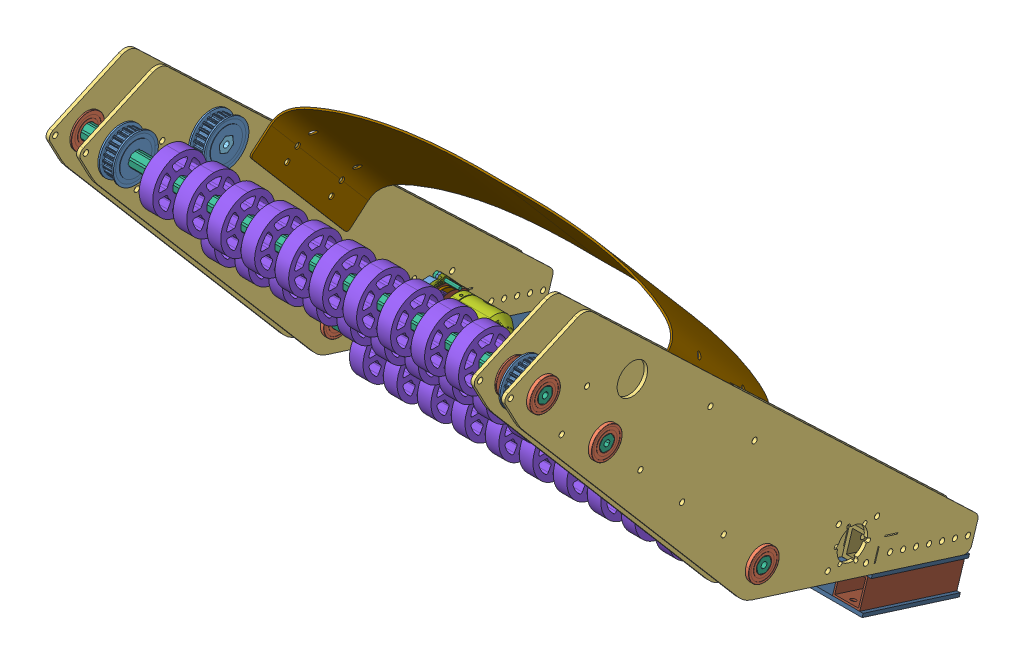
SolidWorks assembly 599-23-Prometheus-IntakeBackup-P-0000, configuration Default. Lengths in mm.
Overall size (438.38 502.65 458.04).
116 component instances, 30 part files, 15 mates.
Components (placement in the parent):
- EBUD-000_INTAKE_STEP_ASM^599-23-Prometheus-IntakeBackup-P-0000-1: EBUD-000_INTAKE_STEP_ASM^599-23-Prometheus-IntakeBackup-P-0000 [Default] at origin size (438.38 502.65 458.04) (virtual)
  - 24T_X_9MM_WIDE_DOUBLE_FLANGE_AL^EBUD-000_INTAKE_STEP_ASM_599-23-Prometheus-IntakeBackup-P-0000-1: 24T_X_9MM_WIDE_DOUBLE_FLANGE_AL^EBUD-000_INTAKE_STEP_ASM_599-23-Prometheus-IntakeBackup-P-0000 [Default] at (-209.55 741.6884 782.7658) x (0 0.711961 0.702219) z (1 0 0) size (42 42 14.5) (virtual)
  - 24T_X_9MM_WIDE_DOUBLE_FLANGE_AL^EBUD-000_INTAKE_STEP_ASM_599-23-Prometheus-IntakeBackup-P-0000-2: 24T_X_9MM_WIDE_DOUBLE_FLANGE_AL^EBUD-000_INTAKE_STEP_ASM_599-23-Prometheus-IntakeBackup-P-0000 [Default] at (-209.55 714.5782 696.9507) x (0 -0.172794 -0.984958) z (1 0 0) size (42 42 14.5) (virtual)
  - 13_75MM__1_2_THUNDERHEX_ID__X_1^EBUD-000_INTAKE_STEP_ASM_599-23-Prometheus-IntakeBackup-P-0000-1: 13_75MM__1_2_THUNDERHEX_ID__X_1^EBUD-000_INTAKE_STEP_ASM_599-23-Prometheus-IntakeBackup-P-0000 [Default] at (-224.6312 714.5782 696.9507) x (0 -0.939164 0.343468) z (1 0 0) size (31.12 31.12 7.94) (virtual)
  - 13_75MM__1_2_THUNDERHEX_ID__X_1^EBUD-000_INTAKE_STEP_ASM_599-23-Prometheus-IntakeBackup-P-0000-2: 13_75MM__1_2_THUNDERHEX_ID__X_1^EBUD-000_INTAKE_STEP_ASM_599-23-Prometheus-IntakeBackup-P-0000 [Default] at (-224.6312 741.6884 782.7658) x (0 -0.292473 -0.956274) z (1 0 0) size (31.12 31.12 7.94) (virtual)
  - 599-23-Prometheus-IntakeBackup-P-0004-1: 599-23-Prometheus-IntakeBackup-P-0004 [Default] at (-223.8375 981.3273 987.2051) x (1 0 0) z (0 -0.649023 0.760769) size (3.17 540.33 141.11)
  - 599-23-Prometheus-IntakeBackup-P-0004-2: 599-23-Prometheus-IntakeBackup-P-0004 [Default] at (-195.2625 981.3273 987.2051) x (1 0 0) z (0 -0.649023 0.760769) size (3.17 540.33 141.11)
  - 599-23-Prometheus-IntakeBackup-P-0004-3: 599-23-Prometheus-IntakeBackup-P-0004 [Default] at (173.1645 981.3273 987.2051) x (1 0 0) z (0 -0.649023 0.760769) size (3.17 540.33 141.11)
  - 599-23-Prometheus-IntakeBackup-P-0004-4: 599-23-Prometheus-IntakeBackup-P-0004 [Default] at (201.7395 981.3273 987.2051) x (1 0 0) z (0 -0.649023 0.760769) size (3.17 540.33 141.11)
  - 13_75MM__1_2_THUNDERHEX_ID__X_1^EBUD-000_INTAKE_STEP_ASM_599-23-Prometheus-IntakeBackup-P-0000-3: 13_75MM__1_2_THUNDERHEX_ID__X_1^EBUD-000_INTAKE_STEP_ASM_599-23-Prometheus-IntakeBackup-P-0000 [Default] at (-194.4688 981.3273 987.2051) x (0 0.254987 0.966944) z (-1 0 0) size (31.12 31.12 7.94) (virtual)
  - 13_75MM__1_2_THUNDERHEX_ID__X_1^EBUD-000_INTAKE_STEP_ASM_599-23-Prometheus-IntakeBackup-P-0000-4: 13_75MM__1_2_THUNDERHEX_ID__X_1^EBUD-000_INTAKE_STEP_ASM_599-23-Prometheus-IntakeBackup-P-0000 [Default] at (-224.6312 950.6568 902.5971) x (0 0.861369 0.50798) z (1 0 0) size (31.12 31.12 7.94) (virtual)
  - 13_75MM__1_2_THUNDERHEX_ID__X_1^EBUD-000_INTAKE_STEP_ASM_599-23-Prometheus-IntakeBackup-P-0000-5: 13_75MM__1_2_THUNDERHEX_ID__X_1^EBUD-000_INTAKE_STEP_ASM_599-23-Prometheus-IntakeBackup-P-0000 [Default] at (-224.6312 981.3273 987.2051) x (0 0.96991 0.243463) z (1 0 0) size (31.12 31.12 7.94) (virtual)
  - 24T_X_9MM_WIDE_DOUBLE_FLANGE_AL^EBUD-000_INTAKE_STEP_ASM_599-23-Prometheus-IntakeBackup-P-0000-3: 24T_X_9MM_WIDE_DOUBLE_FLANGE_AL^EBUD-000_INTAKE_STEP_ASM_599-23-Prometheus-IntakeBackup-P-0000 [Default] at (-183.25 981.3273 987.2051) x (0 -0.068988 0.997618) z (1 0 0) size (42 42 14.5) (virtual)
  - 13_75MM__1_2_THUNDERHEX_ID__X_1^EBUD-000_INTAKE_STEP_ASM_599-23-Prometheus-IntakeBackup-P-0000-6: 13_75MM__1_2_THUNDERHEX_ID__X_1^EBUD-000_INTAKE_STEP_ASM_599-23-Prometheus-IntakeBackup-P-0000 [Default] at (-194.4688 913.695 929.507) x (0 0.294166 0.955754) z (-1 0 0) size (31.12 31.12 7.94) (virtual)
  - 13_75MM__1_2_THUNDERHEX_ID__X_1^EBUD-000_INTAKE_STEP_ASM_599-23-Prometheus-IntakeBackup-P-0000-7: 13_75MM__1_2_THUNDERHEX_ID__X_1^EBUD-000_INTAKE_STEP_ASM_599-23-Prometheus-IntakeBackup-P-0000 [Default] at (-224.6312 913.695 929.507) x (0 0.91904 0.394165) z (1 0 0) size (31.12 31.12 7.94) (virtual)
  - REV-21-1929^EBUD-000_INTAKE_STEP_ASM_599-23-Prometheus-IntakeBackup-P-0000-1: REV-21-1929^EBUD-000_INTAKE_STEP_ASM_599-23-Prometheus-IntakeBackup-P-0000 [Default] at (-209.55 913.695 929.507) x (0 0 1) z (-1 0 0) size (48.2 48.2 12.7) (virtual)
  - 13_75MM__1_2_THUNDERHEX_ID__X_1^EBUD-000_INTAKE_STEP_ASM_599-23-Prometheus-IntakeBackup-P-0000-8: 13_75MM__1_2_THUNDERHEX_ID__X_1^EBUD-000_INTAKE_STEP_ASM_599-23-Prometheus-IntakeBackup-P-0000 [Default] at (-194.4688 741.6884 782.7658) x (0 -0.454664 -0.890663) z (-1 0 0) size (31.12 31.12 7.94) (virtual)
  - REV-21-1929^EBUD-000_INTAKE_STEP_ASM_599-23-Prometheus-IntakeBackup-P-0000-2: REV-21-1929^EBUD-000_INTAKE_STEP_ASM_599-23-Prometheus-IntakeBackup-P-0000 [Default] at (-209.55 950.6568 902.5971) x (0 0.397418 0.917638) z (-1 0 0) size (48.2 48.2 12.7) (virtual)
  - 13_75MM__1_2_THUNDERHEX_ID__X_1^EBUD-000_INTAKE_STEP_ASM_599-23-Prometheus-IntakeBackup-P-0000-9: 13_75MM__1_2_THUNDERHEX_ID__X_1^EBUD-000_INTAKE_STEP_ASM_599-23-Prometheus-IntakeBackup-P-0000 [Default] at (-194.4688 950.6568 902.5971) x (0 0.163432 0.986555) z (-1 0 0) size (31.12 31.12 7.94) (virtual)
  - 24T_X_9MM_WIDE_DOUBLE_FLANGE_AL^EBUD-000_INTAKE_STEP_ASM_599-23-Prometheus-IntakeBackup-P-0000-4: 24T_X_9MM_WIDE_DOUBLE_FLANGE_AL^EBUD-000_INTAKE_STEP_ASM_599-23-Prometheus-IntakeBackup-P-0000 [Default] at (-183.25 950.6568 902.5971) x (0 0.99517 0.098168) z (1 0 0) size (42 42 14.5) (virtual)
  - 13_75MM__1_2_THUNDERHEX_ID__X_1^EBUD-000_INTAKE_STEP_ASM_599-23-Prometheus-IntakeBackup-P-0000-10: 13_75MM__1_2_THUNDERHEX_ID__X_1^EBUD-000_INTAKE_STEP_ASM_599-23-Prometheus-IntakeBackup-P-0000 [Default] at (172.3707 913.695 929.507) x (0 -0.294166 -0.955754) z (1 0 0) size (31.12 31.12 7.94) (virtual)
  - 13_75MM__1_2_THUNDERHEX_ID__X_1^EBUD-000_INTAKE_STEP_ASM_599-23-Prometheus-IntakeBackup-P-0000-11: 13_75MM__1_2_THUNDERHEX_ID__X_1^EBUD-000_INTAKE_STEP_ASM_599-23-Prometheus-IntakeBackup-P-0000 [Default] at (172.3707 741.6884 782.7658) x (0 0.454664 0.890663) z (1 0 0) size (31.12 31.12 7.94) (virtual)
  - 13_75MM__1_2_THUNDERHEX_ID__X_1^EBUD-000_INTAKE_STEP_ASM_599-23-Prometheus-IntakeBackup-P-0000-12: 13_75MM__1_2_THUNDERHEX_ID__X_1^EBUD-000_INTAKE_STEP_ASM_599-23-Prometheus-IntakeBackup-P-0000 [Default] at (202.5333 981.3273 987.2051) x (0 -0.96991 -0.243463) z (-1 0 0) size (31.12 31.12 7.94) (virtual)
  - 13_75MM__1_2_THUNDERHEX_ID__X_1^EBUD-000_INTAKE_STEP_ASM_599-23-Prometheus-IntakeBackup-P-0000-13: 13_75MM__1_2_THUNDERHEX_ID__X_1^EBUD-000_INTAKE_STEP_ASM_599-23-Prometheus-IntakeBackup-P-0000 [Default] at (202.5333 913.695 929.507) x (0 -0.91904 -0.394165) z (-1 0 0) size (31.12 31.12 7.94) (virtual)
  - 13_75MM__1_2_THUNDERHEX_ID__X_1^EBUD-000_INTAKE_STEP_ASM_599-23-Prometheus-IntakeBackup-P-0000-14: 13_75MM__1_2_THUNDERHEX_ID__X_1^EBUD-000_INTAKE_STEP_ASM_599-23-Prometheus-IntakeBackup-P-0000 [Default] at (202.5333 741.6884 782.7658) x (0 0.292473 0.956274) z (-1 0 0) size (31.12 31.12 7.94) (virtual)
  - 13_75MM__1_2_THUNDERHEX_ID__X_1^EBUD-000_INTAKE_STEP_ASM_599-23-Prometheus-IntakeBackup-P-0000-15: 13_75MM__1_2_THUNDERHEX_ID__X_1^EBUD-000_INTAKE_STEP_ASM_599-23-Prometheus-IntakeBackup-P-0000 [Default] at (172.3707 981.3273 987.2051) x (0 -0.254987 -0.966944) z (1 0 0) size (31.12 31.12 7.94) (virtual)
  - 04_CLUSTER_SHAFT^EBUD-000_INTAKE_STEP_ASM_599-23-Prometheus-IntakeBackup-P-0000-1: 04_CLUSTER_SHAFT^EBUD-000_INTAKE_STEP_ASM_599-23-Prometheus-IntakeBackup-P-0000 [Default] at (-190.605 950.6568 902.5971) x (1 0 0) z (0 0.754856 0.65589) size (55.88 13.76 12.7) (virtual)
  - 24T_X_9MM_WIDE_DOUBLE_FLANGE_AL^EBUD-000_INTAKE_STEP_ASM_599-23-Prometheus-IntakeBackup-P-0000-5: 24T_X_9MM_WIDE_DOUBLE_FLANGE_AL^EBUD-000_INTAKE_STEP_ASM_599-23-Prometheus-IntakeBackup-P-0000 [Default] at (191.3145 741.6884 782.7658) x (0 -0.01901 0.999819) z (1 0 0) size (42 42 14.5) (virtual)
  - 24T_X_9MM_WIDE_DOUBLE_FLANGE_AL^EBUD-000_INTAKE_STEP_ASM_599-23-Prometheus-IntakeBackup-P-0000-6: 24T_X_9MM_WIDE_DOUBLE_FLANGE_AL^EBUD-000_INTAKE_STEP_ASM_599-23-Prometheus-IntakeBackup-P-0000 [Default] at (191.3145 981.3273 987.2051) x (0 -0.068988 0.997618) z (1 0 0) size (42 42 14.5) (virtual)
  - 04_INTAKE_ROLLER_SHAFT^EBUD-000_INTAKE_STEP_ASM_599-23-Prometheus-IntakeBackup-P-0000-1: 04_INTAKE_ROLLER_SHAFT^EBUD-000_INTAKE_STEP_ASM_599-23-Prometheus-IntakeBackup-P-0000 [Default] at (-37.973 741.6873 782.7662) x (1 0 0) z (0 -0.958269 0.285869) size (435.1 13.76 12.7) (virtual)
  - 04_INTAKE_ROLLER_SHAFT^EBUD-000_INTAKE_STEP_ASM_599-23-Prometheus-IntakeBackup-P-0000-2: 04_INTAKE_ROLLER_SHAFT^EBUD-000_INTAKE_STEP_ASM_599-23-Prometheus-IntakeBackup-P-0000 [Default] at (-37.973 913.695 929.507) x (1 0 0) z (0 -0.53426 -0.84532) size (435.1 13.76 12.7) (virtual)
  - 04_INTAKE_ROLLER_SHAFT^EBUD-000_INTAKE_STEP_ASM_599-23-Prometheus-IntakeBackup-P-0000-3: 04_INTAKE_ROLLER_SHAFT^EBUD-000_INTAKE_STEP_ASM_599-23-Prometheus-IntakeBackup-P-0000 [Default] at (-37.973 981.3273 987.2051) size (435.1 13.76 12.7) (virtual)
- REV_ULTRAPLANETARY_1-STAGE_ASM^599-23-Prometheus-IntakeBackup-P-0000-1: REV_ULTRAPLANETARY_1-STAGE_ASM^599-23-Prometheus-IntakeBackup-P-0000 [Default] at (-167.425 714.5782 696.9507) x (0 -0.976417 -0.215894) z (1 0 0) size (56.74 54.7 105.61) (virtual)
  - REV_ULTRAPLANETARY__CONFIGURABL_ASM^REV_ULTRAPLANETARY_1-STAGE_ASM_599-23-Prometheus-IntakeBackup-P-0000-1: REV_ULTRAPLANETARY__CONFIGURABL_ASM^REV_ULTRAPLANETARY_1-STAGE_ASM_599-23-Prometheus-IntakeBackup-P-0000 [Default] at origin size (56.74 54.7 105.61) (virtual)
    - REV_PLANETARY_STAGE__1__ASM^REV_ULTRAPLANETARY__CONFIGURABL_ASM_REV_ULTRAPLANETARY_1-STAGE_ASM_599-23-Prometheus-IntakeBackup-P-0000-1: REV_PLANETARY_STAGE__1__ASM^REV_ULTRAPLANETARY__CONFIGURABL_ASM_REV_ULTRAPLANETARY_1-STAGE_ASM_599-23-Prometheus-IntakeBackup-P-0000 [Default] at origin size (47.64 47.49 16.75) (virtual)
      - REV_ULTRAPLANETARY_3_1_CARTRIDG_ASM^REV_PLANETARY_STAGE__1__ASM_REV_ULTRAPLANETARY__CONFIGURABL_ASM_REV_ULTRAPLANETARY_1-STAGE_ASM_599-23-Prometheus-IntakeBackup-P-0000-1: REV_ULTRAPLANETARY_3_1_CARTRIDG_ASM^REV_PLANETARY_STAGE__1__ASM_REV_ULTRAPLANETARY__CONFIGURABL_ASM_REV_ULTRAPLANETARY_1-STAGE_ASM_599-23-Prometheus-IntakeBackup-P-0000 [Default] at origin size (47.64 47.49 16.75) (virtual)
        - REV-40-1613^REV_ULTRAPLANETARY_3_1_CARTRIDG_ASM_REV_PLANETARY_STAGE__1__ASM_REV_ULTRAPLANETARY__CONFIGURABL_ASM_REV_ULTRAPLANETARY_1-STAGE_ASM_599-23-Prometheus-IntakeBackup-P-0000-1: REV-40-1613^REV_ULTRAPLANETARY_3_1_CARTRIDG_ASM_REV_PLANETARY_STAGE__1__ASM_REV_ULTRAPLANETARY__CONFIGURABL_ASM_REV_ULTRAPLANETARY_1-STAGE_ASM_599-23-Prometheus-IntakeBackup-P-0000 [Default] at (-0.89 11.5157 -14.625) x (0 0 1) z (-0.923728 -0.383049 0) size (9 3 3) (virtual)
        - REV-41-1601-2^REV_ULTRAPLANETARY_3_1_CARTRIDG_ASM_REV_PLANETARY_STAGE__1__ASM_REV_ULTRAPLANETARY__CONFIGURABL_ASM_REV_ULTRAPLANETARY_1-STAGE_ASM_599-23-Prometheus-IntakeBackup-P-0000-1: REV-41-1601-2^REV_ULTRAPLANETARY_3_1_CARTRIDG_ASM_REV_PLANETARY_STAGE__1__ASM_REV_ULTRAPLANETARY__CONFIGURABL_ASM_REV_ULTRAPLANETARY_1-STAGE_ASM_599-23-Prometheus-IntakeBackup-P-0000 [Default] at (-0.89 11.5157 -8.625) x (0.281273 0.959628 0) z (0.959628 -0.281273 0) size (8.22 6.01 8.17) (virtual)
        - REV-41-1601-2^REV_ULTRAPLANETARY_3_1_CARTRIDG_ASM_REV_PLANETARY_STAGE__1__ASM_REV_ULTRAPLANETARY__CONFIGURABL_ASM_REV_ULTRAPLANETARY_1-STAGE_ASM_599-23-Prometheus-IntakeBackup-P-0000-2: REV-41-1601-2^REV_ULTRAPLANETARY_3_1_CARTRIDG_ASM_REV_PLANETARY_STAGE__1__ASM_REV_ULTRAPLANETARY__CONFIGURABL_ASM_REV_ULTRAPLANETARY_1-STAGE_ASM_599-23-Prometheus-IntakeBackup-P-0000 [Default] at (-11.5157 -0.89 -8.625) x (0.938661 0.34484 0) z (0.34484 -0.938661 0) size (8.22 6.01 8.17) (virtual)
        - REV-40-1613^REV_ULTRAPLANETARY_3_1_CARTRIDG_ASM_REV_PLANETARY_STAGE__1__ASM_REV_ULTRAPLANETARY__CONFIGURABL_ASM_REV_ULTRAPLANETARY_1-STAGE_ASM_599-23-Prometheus-IntakeBackup-P-0000-2: REV-40-1613^REV_ULTRAPLANETARY_3_1_CARTRIDG_ASM_REV_PLANETARY_STAGE__1__ASM_REV_ULTRAPLANETARY__CONFIGURABL_ASM_REV_ULTRAPLANETARY_1-STAGE_ASM_599-23-Prometheus-IntakeBackup-P-0000 [Default] at (0.89 -11.5157 -14.625) x (0 0 1) z (-0.923728 -0.383049 0) size (9 3 3) (virtual)
        - REV-40-1613^REV_ULTRAPLANETARY_3_1_CARTRIDG_ASM_REV_PLANETARY_STAGE__1__ASM_REV_ULTRAPLANETARY__CONFIGURABL_ASM_REV_ULTRAPLANETARY_1-STAGE_ASM_599-23-Prometheus-IntakeBackup-P-0000-3: REV-40-1613^REV_ULTRAPLANETARY_3_1_CARTRIDG_ASM_REV_PLANETARY_STAGE__1__ASM_REV_ULTRAPLANETARY__CONFIGURABL_ASM_REV_ULTRAPLANETARY_1-STAGE_ASM_599-23-Prometheus-IntakeBackup-P-0000 [Default] at (11.5157 0.89 -14.625) x (0 0 1) z (-0.923728 -0.383049 0) size (9 3 3) (virtual)
        - REV-41-1601-1^REV_ULTRAPLANETARY_3_1_CARTRIDG_ASM_REV_PLANETARY_STAGE__1__ASM_REV_ULTRAPLANETARY__CONFIGURABL_ASM_REV_ULTRAPLANETARY_1-STAGE_ASM_599-23-Prometheus-IntakeBackup-P-0000-1: REV-41-1601-1^REV_ULTRAPLANETARY_3_1_CARTRIDG_ASM_REV_PLANETARY_STAGE__1__ASM_REV_ULTRAPLANETARY__CONFIGURABL_ASM_REV_ULTRAPLANETARY_1-STAGE_ASM_599-23-Prometheus-IntakeBackup-P-0000 [Default] at (0 0 -11.875) x (0.997027 0.077058 0) z (0 0 -1) size (29.1 29.1 10.25) (virtual)
        - REV-41-1601-2^REV_ULTRAPLANETARY_3_1_CARTRIDG_ASM_REV_PLANETARY_STAGE__1__ASM_REV_ULTRAPLANETARY__CONFIGURABL_ASM_REV_ULTRAPLANETARY_1-STAGE_ASM_599-23-Prometheus-IntakeBackup-P-0000-3: REV-41-1601-2^REV_ULTRAPLANETARY_3_1_CARTRIDG_ASM_REV_PLANETARY_STAGE__1__ASM_REV_ULTRAPLANETARY__CONFIGURABL_ASM_REV_ULTRAPLANETARY_1-STAGE_ASM_599-23-Prometheus-IntakeBackup-P-0000 [Default] at (0.89 -11.5157 -8.625) x (0.79716 -0.603767 0) z (-0.603767 -0.79716 0) size (8.22 6.01 8.17) (virtual)
        - REV-41-1601-3^REV_ULTRAPLANETARY_3_1_CARTRIDG_ASM_REV_PLANETARY_STAGE__1__ASM_REV_ULTRAPLANETARY__CONFIGURABL_ASM_REV_ULTRAPLANETARY_1-STAGE_ASM_599-23-Prometheus-IntakeBackup-P-0000-1: REV-41-1601-3^REV_ULTRAPLANETARY_3_1_CARTRIDG_ASM_REV_PLANETARY_STAGE__1__ASM_REV_ULTRAPLANETARY__CONFIGURABL_ASM_REV_ULTRAPLANETARY_1-STAGE_ASM_599-23-Prometheus-IntakeBackup-P-0000 [Default] at (0 0 -8.75) x (-0.670912 -0.741537 0) z (-0.741537 0.670912 0) size (17.04 6.01 17.02) (virtual)
        - REV-40-1619^REV_ULTRAPLANETARY_3_1_CARTRIDG_ASM_REV_PLANETARY_STAGE__1__ASM_REV_ULTRAPLANETARY__CONFIGURABL_ASM_REV_ULTRAPLANETARY_1-STAGE_ASM_599-23-Prometheus-IntakeBackup-P-0000-1: REV-40-1619^REV_ULTRAPLANETARY_3_1_CARTRIDG_ASM_REV_PLANETARY_STAGE__1__ASM_REV_ULTRAPLANETARY__CONFIGURABL_ASM_REV_ULTRAPLANETARY_1-STAGE_ASM_599-23-Prometheus-IntakeBackup-P-0000 [Default] at (0 0 -14.875) x (-0.866025 -0.5 0) z (0 0 -1) size (35.02 34.62 3.62) (virtual)
        - REV-40-1619^REV_ULTRAPLANETARY_3_1_CARTRIDG_ASM_REV_PLANETARY_STAGE__1__ASM_REV_ULTRAPLANETARY__CONFIGURABL_ASM_REV_ULTRAPLANETARY_1-STAGE_ASM_599-23-Prometheus-IntakeBackup-P-0000-2: REV-40-1619^REV_ULTRAPLANETARY_3_1_CARTRIDG_ASM_REV_PLANETARY_STAGE__1__ASM_REV_ULTRAPLANETARY__CONFIGURABL_ASM_REV_ULTRAPLANETARY_1-STAGE_ASM_599-23-Prometheus-IntakeBackup-P-0000 [Default] at (0 0 -5.125) x (0 -1 0) z (0 0 1) size (35.02 34.62 3.62) (virtual)
        - REV-40-1613^REV_ULTRAPLANETARY_3_1_CARTRIDG_ASM_REV_PLANETARY_STAGE__1__ASM_REV_ULTRAPLANETARY__CONFIGURABL_ASM_REV_ULTRAPLANETARY_1-STAGE_ASM_599-23-Prometheus-IntakeBackup-P-0000-4: REV-40-1613^REV_ULTRAPLANETARY_3_1_CARTRIDG_ASM_REV_PLANETARY_STAGE__1__ASM_REV_ULTRAPLANETARY__CONFIGURABL_ASM_REV_ULTRAPLANETARY_1-STAGE_ASM_599-23-Prometheus-IntakeBackup-P-0000 [Default] at (-11.5157 -0.89 -14.625) x (0 0 1) z (-0.923728 -0.383049 0) size (9 3 3) (virtual)
        - REV-41-1601-2^REV_ULTRAPLANETARY_3_1_CARTRIDG_ASM_REV_PLANETARY_STAGE__1__ASM_REV_ULTRAPLANETARY__CONFIGURABL_ASM_REV_ULTRAPLANETARY_1-STAGE_ASM_599-23-Prometheus-IntakeBackup-P-0000-4: REV-41-1601-2^REV_ULTRAPLANETARY_3_1_CARTRIDG_ASM_REV_PLANETARY_STAGE__1__ASM_REV_ULTRAPLANETARY__CONFIGURABL_ASM_REV_ULTRAPLANETARY_1-STAGE_ASM_599-23-Prometheus-IntakeBackup-P-0000 [Default] at (11.5157 0.89 -8.625) x (0.79726 -0.603636 0) z (-0.603636 -0.79726 0) size (8.22 6.01 8.17) (virtual)
    - REV_ULTRAPLANETARY_OUTPUT_STAGE_ASM^REV_ULTRAPLANETARY__CONFIGURABL_ASM_REV_ULTRAPLANETARY_1-STAGE_ASM_599-23-Prometheus-IntakeBackup-P-0000-1: REV_ULTRAPLANETARY_OUTPUT_STAGE_ASM^REV_ULTRAPLANETARY__CONFIGURABL_ASM_REV_ULTRAPLANETARY_1-STAGE_ASM_599-23-Prometheus-IntakeBackup-P-0000 [Default] at origin size (56.74 54.7 18.3) (virtual)
      - REV-41-1604-5^REV_ULTRAPLANETARY_OUTPUT_STAGE_ASM_REV_ULTRAPLANETARY__CONFIGURABL_ASM_REV_ULTRAPLANETARY_1-STAGE_ASM_599-23-Prometheus-IntakeBackup-P-0000-1: REV-41-1604-5^REV_ULTRAPLANETARY_OUTPUT_STAGE_ASM_REV_ULTRAPLANETARY__CONFIGURABL_ASM_REV_ULTRAPLANETARY_1-STAGE_ASM_599-23-Prometheus-IntakeBackup-P-0000 [Default] at (0 0 -21.25) x (0.103978 -0.99458 0) z (0.99458 0.103978 0) size (23.5 0.75 23.5) (virtual)
      - SOCKET_HEAD_CAP_SCREW_AM_B18_3_^REV_ULTRAPLANETARY_OUTPUT_STAGE_ASM_REV_ULTRAPLANETARY__CONFIGURABL_ASM_REV_ULTRAPLANETARY_1-STAGE_ASM_599-23-Prometheus-IntakeBackup-P-0000-1: SOCKET_HEAD_CAP_SCREW_AM_B18_3_^REV_ULTRAPLANETARY_OUTPUT_STAGE_ASM_REV_ULTRAPLANETARY__CONFIGURABL_ASM_REV_ULTRAPLANETARY_1-STAGE_ASM_599-23-Prometheus-IntakeBackup-P-0000 [Default] at (15.6357 3.3948 -15.05) x (0 0 -1) z (-0.934724 -0.355374 0) size (6 3.8 3.8) (virtual)
      - MCMASTER-CARR_91292A004_91292A0^REV_ULTRAPLANETARY_OUTPUT_STAGE_ASM_REV_ULTRAPLANETARY__CONFIGURABL_ASM_REV_ULTRAPLANETARY_1-STAGE_ASM_599-23-Prometheus-IntakeBackup-P-0000-1: MCMASTER-CARR_91292A004_91292A0^REV_ULTRAPLANETARY_OUTPUT_STAGE_ASM_REV_ULTRAPLANETARY__CONFIGURABL_ASM_REV_ULTRAPLANETARY_1-STAGE_ASM_599-23-Prometheus-IntakeBackup-P-0000 [Default] at (-3.715 6.4346 -21.5) x (-0.608447 -0.793594 0) z (-0.793594 0.608447 0) size (3.8 6 3.8) (virtual)
      - 6704ZZ^REV_ULTRAPLANETARY_OUTPUT_STAGE_ASM_REV_ULTRAPLANETARY__CONFIGURABL_ASM_REV_ULTRAPLANETARY_1-STAGE_ASM_599-23-Prometheus-IntakeBackup-P-0000-1: 6704ZZ^REV_ULTRAPLANETARY_OUTPUT_STAGE_ASM_REV_ULTRAPLANETARY__CONFIGURABL_ASM_REV_ULTRAPLANETARY_1-STAGE_ASM_599-23-Prometheus-IntakeBackup-P-0000 [Default] at (0 0 -23.25) x (0.117109 -0.993119 0) z (0.993119 0.117109 0) size (27 4 27) (virtual)
      - 6704ZZ^REV_ULTRAPLANETARY_OUTPUT_STAGE_ASM_REV_ULTRAPLANETARY__CONFIGURABL_ASM_REV_ULTRAPLANETARY_1-STAGE_ASM_599-23-Prometheus-IntakeBackup-P-0000-2: 6704ZZ^REV_ULTRAPLANETARY_OUTPUT_STAGE_ASM_REV_ULTRAPLANETARY__CONFIGURABL_ASM_REV_ULTRAPLANETARY_1-STAGE_ASM_599-23-Prometheus-IntakeBackup-P-0000 [Default] at (0 0 -18.5) x (-0.099871 -0.995 0) z (0.995 -0.099871 0) size (27 4 27) (virtual)
      - MCMASTER-CARR_91292A004_91292A0^REV_ULTRAPLANETARY_OUTPUT_STAGE_ASM_REV_ULTRAPLANETARY__CONFIGURABL_ASM_REV_ULTRAPLANETARY_1-STAGE_ASM_599-23-Prometheus-IntakeBackup-P-0000-2: MCMASTER-CARR_91292A004_91292A0^REV_ULTRAPLANETARY_OUTPUT_STAGE_ASM_REV_ULTRAPLANETARY__CONFIGURABL_ASM_REV_ULTRAPLANETARY_1-STAGE_ASM_599-23-Prometheus-IntakeBackup-P-0000 [Default] at (-3.715 -6.4346 -21.5) x (0.991496 -0.130134 0) z (-0.130134 -0.991496 0) size (3.8 6 3.8) (virtual)
      - MCMASTER-CARR_91292A004_91292A0^REV_ULTRAPLANETARY_OUTPUT_STAGE_ASM_REV_ULTRAPLANETARY__CONFIGURABL_ASM_REV_ULTRAPLANETARY_1-STAGE_ASM_599-23-Prometheus-IntakeBackup-P-0000-3: MCMASTER-CARR_91292A004_91292A0^REV_ULTRAPLANETARY_OUTPUT_STAGE_ASM_REV_ULTRAPLANETARY__CONFIGURABL_ASM_REV_ULTRAPLANETARY_1-STAGE_ASM_599-23-Prometheus-IntakeBackup-P-0000 [Default] at (7.43 0 -21.5) x (-0.383049 0.923728 0) z (0.923728 0.383049 0) size (3.8 6 3.8) (virtual)
      - SOCKET_HEAD_CAP_SCREW_AM_B18_3_^REV_ULTRAPLANETARY_OUTPUT_STAGE_ASM_REV_ULTRAPLANETARY__CONFIGURABL_ASM_REV_ULTRAPLANETARY_1-STAGE_ASM_599-23-Prometheus-IntakeBackup-P-0000-2: SOCKET_HEAD_CAP_SCREW_AM_B18_3_^REV_ULTRAPLANETARY_OUTPUT_STAGE_ASM_REV_ULTRAPLANETARY__CONFIGURABL_ASM_REV_ULTRAPLANETARY_1-STAGE_ASM_599-23-Prometheus-IntakeBackup-P-0000 [Default] at (-10.7579 11.8435 -15.05) x (0 0 -1) z (-0.492915 -0.870077 0) size (6 3.8 3.8) (virtual)
      - REV-41-1604-2^REV_ULTRAPLANETARY_OUTPUT_STAGE_ASM_REV_ULTRAPLANETARY__CONFIGURABL_ASM_REV_ULTRAPLANETARY_1-STAGE_ASM_599-23-Prometheus-IntakeBackup-P-0000-1: REV-41-1604-2^REV_ULTRAPLANETARY_OUTPUT_STAGE_ASM_REV_ULTRAPLANETARY__CONFIGURABL_ASM_REV_ULTRAPLANETARY_1-STAGE_ASM_599-23-Prometheus-IntakeBackup-P-0000 [Default] at (0 0 -26.25) x (0 -1 0) z (1 0 0) size (43.57 6.3 38.01) (virtual)
      - REV-41-1611_THROUGH_HOLE^REV_ULTRAPLANETARY_OUTPUT_STAGE_ASM_REV_ULTRAPLANETARY__CONFIGURABL_ASM_REV_ULTRAPLANETARY_1-STAGE_ASM_599-23-Prometheus-IntakeBackup-P-0000-1: REV-41-1611_THROUGH_HOLE^REV_ULTRAPLANETARY_OUTPUT_STAGE_ASM_REV_ULTRAPLANETARY__CONFIGURABL_ASM_REV_ULTRAPLANETARY_1-STAGE_ASM_599-23-Prometheus-IntakeBackup-P-0000 [Default] at (0 0 -15.25) x (0 1 0) z (1 0 0) size (22 6.76 22) (virtual)
      - REV-41-1612^REV_ULTRAPLANETARY_OUTPUT_STAGE_ASM_REV_ULTRAPLANETARY__CONFIGURABL_ASM_REV_ULTRAPLANETARY_1-STAGE_ASM_599-23-Prometheus-IntakeBackup-P-0000-1: REV-41-1612^REV_ULTRAPLANETARY_OUTPUT_STAGE_ASM_REV_ULTRAPLANETARY__CONFIGURABL_ASM_REV_ULTRAPLANETARY_1-STAGE_ASM_599-23-Prometheus-IntakeBackup-P-0000 [Default] at (0 0 -19) x (-0.5 -0.866025 0) z (0 0 -1) size (22 21.65 13.25) (virtual)
      - REV-41-1604-1^REV_ULTRAPLANETARY_OUTPUT_STAGE_ASM_REV_ULTRAPLANETARY__CONFIGURABL_ASM_REV_ULTRAPLANETARY_1-STAGE_ASM_599-23-Prometheus-IntakeBackup-P-0000-1: REV-41-1604-1^REV_ULTRAPLANETARY_OUTPUT_STAGE_ASM_REV_ULTRAPLANETARY__CONFIGURABL_ASM_REV_ULTRAPLANETARY_1-STAGE_ASM_599-23-Prometheus-IntakeBackup-P-0000 [Default] at (0 0 -19.25) x (0.866025 -0.5 0) z (-0.5 -0.866025 0) size (43.57 7.04 38.01) (virtual)
      - SOCKET_HEAD_CAP_SCREW_AM_B18_3_^REV_ULTRAPLANETARY_OUTPUT_STAGE_ASM_REV_ULTRAPLANETARY__CONFIGURABL_ASM_REV_ULTRAPLANETARY_1-STAGE_ASM_599-23-Prometheus-IntakeBackup-P-0000-3: SOCKET_HEAD_CAP_SCREW_AM_B18_3_^REV_ULTRAPLANETARY_OUTPUT_STAGE_ASM_REV_ULTRAPLANETARY__CONFIGURABL_ASM_REV_ULTRAPLANETARY_1-STAGE_ASM_599-23-Prometheus-IntakeBackup-P-0000 [Default] at (-4.8778 -15.2383 -15.05) x (0 0 -1) z (0.970727 -0.240185 0) size (6 3.8 3.8) (virtual)
    - REV_ULTRAPLANETARY_550_MOTOR_PL_ASM^REV_ULTRAPLANETARY__CONFIGURABL_ASM_REV_ULTRAPLANETARY_1-STAGE_ASM_599-23-Prometheus-IntakeBackup-P-0000-1: REV_ULTRAPLANETARY_550_MOTOR_PL_ASM^REV_ULTRAPLANETARY__CONFIGURABL_ASM_REV_ULTRAPLANETARY_1-STAGE_ASM_599-23-Prometheus-IntakeBackup-P-0000 [Default] at origin size (9.12 31.6 16.65) (virtual)
      - REV-41-1608^REV_ULTRAPLANETARY_550_MOTOR_PL_ASM_REV_ULTRAPLANETARY__CONFIGURABL_ASM_REV_ULTRAPLANETARY_1-STAGE_ASM_599-23-Prometheus-IntakeBackup-P-0000-1: REV-41-1608^REV_ULTRAPLANETARY_550_MOTOR_PL_ASM_REV_ULTRAPLANETARY__CONFIGURABL_ASM_REV_ULTRAPLANETARY_1-STAGE_ASM_599-23-Prometheus-IntakeBackup-P-0000 [Default] at (0 0 -8) x (-0.123066 0.992399 0) z (0.992399 0.123066 0) size (8.22 7 8.17) (virtual)
      - M3X8_BUTTON_HEAD_91239A113^REV_ULTRAPLANETARY_550_MOTOR_PL_ASM_REV_ULTRAPLANETARY__CONFIGURABL_ASM_REV_ULTRAPLANETARY_1-STAGE_ASM_599-23-Prometheus-IntakeBackup-P-0000-1: M3X8_BUTTON_HEAD_91239A113^REV_ULTRAPLANETARY_550_MOTOR_PL_ASM_REV_ULTRAPLANETARY__CONFIGURABL_ASM_REV_ULTRAPLANETARY_1-STAGE_ASM_599-23-Prometheus-IntakeBackup-P-0000 [Default] at (0.5 -12.49 -4.5) x (-0.04 0.9992 0) z (0.9992 0.04 0) size (5.7 9.66 5.7) (virtual)
      - M3X8_BUTTON_HEAD_91239A113^REV_ULTRAPLANETARY_550_MOTOR_PL_ASM_REV_ULTRAPLANETARY__CONFIGURABL_ASM_REV_ULTRAPLANETARY_1-STAGE_ASM_599-23-Prometheus-IntakeBackup-P-0000-2: M3X8_BUTTON_HEAD_91239A113^REV_ULTRAPLANETARY_550_MOTOR_PL_ASM_REV_ULTRAPLANETARY__CONFIGURABL_ASM_REV_ULTRAPLANETARY_1-STAGE_ASM_599-23-Prometheus-IntakeBackup-P-0000 [Default] at (-0.5 12.49 -4.5) x (-0.938759 0.344575 0) z (0.344575 0.938759 0) size (5.7 9.66 5.7) (virtual)
    - HEX_SOCKET_HEAD_CAP_SCREW_M3X0_^REV_ULTRAPLANETARY__CONFIGURABL_ASM_REV_ULTRAPLANETARY_1-STAGE_ASM_599-23-Prometheus-IntakeBackup-P-0000-1: HEX_SOCKET_HEAD_CAP_SCREW_M3X0_^REV_ULTRAPLANETARY__CONFIGURABL_ASM_REV_ULTRAPLANETARY_1-STAGE_ASM_599-23-Prometheus-IntakeBackup-P-0000 [Default] at (6.9282 4 -38.25) x (-0.866025 0.5 0) z (0 0 -1) size (5.5 5.5 11) (virtual)
    - HEX_SOCKET_HEAD_CAP_SCREW_M3X0_^REV_ULTRAPLANETARY__CONFIGURABL_ASM_REV_ULTRAPLANETARY_1-STAGE_ASM_599-23-Prometheus-IntakeBackup-P-0000-2: HEX_SOCKET_HEAD_CAP_SCREW_M3X0_^REV_ULTRAPLANETARY__CONFIGURABL_ASM_REV_ULTRAPLANETARY_1-STAGE_ASM_599-23-Prometheus-IntakeBackup-P-0000 [Default] at (0 8 -38.25) x (-0.866025 -0.5 0) z (0 0 -1) size (5.5 5.5 11) (virtual)
    - UP_1_2__HEX_ADAPTER__REV-41-162^REV_ULTRAPLANETARY__CONFIGURABL_ASM_REV_ULTRAPLANETARY_1-STAGE_ASM_599-23-Prometheus-IntakeBackup-P-0000-1: UP_1_2__HEX_ADAPTER__REV-41-162^REV_ULTRAPLANETARY__CONFIGURABL_ASM_REV_ULTRAPLANETARY_1-STAGE_ASM_599-23-Prometheus-IntakeBackup-P-0000 [Default] at (0 0 -32.25) x (-0.5 -0.866025 0) z (0 0 1) size (22 22 30.59) (virtual)
    - HEX_SOCKET_HEAD_CAP_SCREW_M3X0_^REV_ULTRAPLANETARY__CONFIGURABL_ASM_REV_ULTRAPLANETARY_1-STAGE_ASM_599-23-Prometheus-IntakeBackup-P-0000-3: HEX_SOCKET_HEAD_CAP_SCREW_M3X0_^REV_ULTRAPLANETARY__CONFIGURABL_ASM_REV_ULTRAPLANETARY_1-STAGE_ASM_599-23-Prometheus-IntakeBackup-P-0000 [Default] at (0 -8 -38.25) x (0.866025 0.5 0) z (0 0 -1) size (5.5 5.5 11) (virtual)
    - HEX_SOCKET_HEAD_CAP_SCREW_M3X0_^REV_ULTRAPLANETARY__CONFIGURABL_ASM_REV_ULTRAPLANETARY_1-STAGE_ASM_599-23-Prometheus-IntakeBackup-P-0000-4: HEX_SOCKET_HEAD_CAP_SCREW_M3X0_^REV_ULTRAPLANETARY__CONFIGURABL_ASM_REV_ULTRAPLANETARY_1-STAGE_ASM_599-23-Prometheus-IntakeBackup-P-0000 [Default] at (-6.9282 -4 -38.25) x (0.866025 -0.5 0) z (0 0 -1) size (5.5 5.5 11) (virtual)
    - M3X40_91290A136^REV_ULTRAPLANETARY__CONFIGURABL_ASM_REV_ULTRAPLANETARY_1-STAGE_ASM_599-23-Prometheus-IntakeBackup-P-0000-1: M3X40_91290A136^REV_ULTRAPLANETARY__CONFIGURABL_ASM_REV_ULTRAPLANETARY_1-STAGE_ASM_599-23-Prometheus-IntakeBackup-P-0000 [Default] at (0 18.4752 18.75) x (-0.866025 0.5 0) z (-0.5 -0.866025 0) size (5.5 23.01 5.5) (virtual)
    - M3X40_91290A136^REV_ULTRAPLANETARY__CONFIGURABL_ASM_REV_ULTRAPLANETARY_1-STAGE_ASM_599-23-Prometheus-IntakeBackup-P-0000-2: M3X40_91290A136^REV_ULTRAPLANETARY__CONFIGURABL_ASM_REV_ULTRAPLANETARY_1-STAGE_ASM_599-23-Prometheus-IntakeBackup-P-0000 [Default] at (-16 9.2376 18.75) x (-0.866025 -0.5 0) z (0.5 -0.866025 0) size (5.5 23.01 5.5) (virtual)
    - M3X40_91290A136^REV_ULTRAPLANETARY__CONFIGURABL_ASM_REV_ULTRAPLANETARY_1-STAGE_ASM_599-23-Prometheus-IntakeBackup-P-0000-3: M3X40_91290A136^REV_ULTRAPLANETARY__CONFIGURABL_ASM_REV_ULTRAPLANETARY_1-STAGE_ASM_599-23-Prometheus-IntakeBackup-P-0000 [Default] at (16 -9.2376 18.75) x (0.866025 0.5 0) z (-0.5 0.866025 0) size (5.5 23.01 5.5) (virtual)
    - HEX_SOCKET_HEAD_CAP_SCREW_M3X0_^REV_ULTRAPLANETARY__CONFIGURABL_ASM_REV_ULTRAPLANETARY_1-STAGE_ASM_599-23-Prometheus-IntakeBackup-P-0000-5: HEX_SOCKET_HEAD_CAP_SCREW_M3X0_^REV_ULTRAPLANETARY__CONFIGURABL_ASM_REV_ULTRAPLANETARY_1-STAGE_ASM_599-23-Prometheus-IntakeBackup-P-0000 [Default] at (6.9282 -4 -38.25) x (0 1 0) z (0 0 -1) size (5.5 5.5 11) (virtual)
    - M3X40_91290A136^REV_ULTRAPLANETARY__CONFIGURABL_ASM_REV_ULTRAPLANETARY_1-STAGE_ASM_599-23-Prometheus-IntakeBackup-P-0000-4: M3X40_91290A136^REV_ULTRAPLANETARY__CONFIGURABL_ASM_REV_ULTRAPLANETARY_1-STAGE_ASM_599-23-Prometheus-IntakeBackup-P-0000 [Default] at (-16 -9.2376 18.75) x (0 -1 0) z (1 0 0) size (5.5 23.01 5.5) (virtual)
    - M3X40_91290A136^REV_ULTRAPLANETARY__CONFIGURABL_ASM_REV_ULTRAPLANETARY_1-STAGE_ASM_599-23-Prometheus-IntakeBackup-P-0000-5: M3X40_91290A136^REV_ULTRAPLANETARY__CONFIGURABL_ASM_REV_ULTRAPLANETARY_1-STAGE_ASM_599-23-Prometheus-IntakeBackup-P-0000 [Default] at (0 -18.4752 18.75) x (0.866025 -0.5 0) z (0.5 0.866025 0) size (5.5 23.01 5.5) (virtual)
    - M3X40_91290A136^REV_ULTRAPLANETARY__CONFIGURABL_ASM_REV_ULTRAPLANETARY_1-STAGE_ASM_599-23-Prometheus-IntakeBackup-P-0000-6: M3X40_91290A136^REV_ULTRAPLANETARY__CONFIGURABL_ASM_REV_ULTRAPLANETARY_1-STAGE_ASM_599-23-Prometheus-IntakeBackup-P-0000 [Default] at (16 9.2376 18.75) x (0 1 0) z (-1 0 0) size (5.5 23.01 5.5) (virtual)
    - NEO_550_MOTOR__REV-21-1651_^REV_ULTRAPLANETARY__CONFIGURABL_ASM_REV_ULTRAPLANETARY_1-STAGE_ASM_599-23-Prometheus-IntakeBackup-P-0000-1: NEO_550_MOTOR__REV-21-1651_^REV_ULTRAPLANETARY__CONFIGURABL_ASM_REV_ULTRAPLANETARY_1-STAGE_ASM_599-23-Prometheus-IntakeBackup-P-0000 [Default] at (0 0 -11.5) x (0 0 1) z (-1 0 0) size (56.02 43 42.91) (virtual)
- TTB-0032_2INCH_SQUISH_WHEEL^599-23-Prometheus-IntakeBackup-P-0000-1: TTB-0032_2INCH_SQUISH_WHEEL^599-23-Prometheus-IntakeBackup-P-0000 [Default] at (143.002 741.6873 782.7662) x (0 0.999841 0.017831) z (0 -0.017831 0.999841) size (50.8 12.7 50.8) (virtual)
- TTB-0032_2INCH_SQUISH_WHEEL^599-23-Prometheus-IntakeBackup-P-0000-2: TTB-0032_2INCH_SQUISH_WHEEL^599-23-Prometheus-IntakeBackup-P-0000 [Default] at (111.252 741.6873 782.7662) x (0 0.999841 0.017831) z (0 -0.017831 0.999841) size (50.8 12.7 50.8) (virtual)
- TTB-0032_2INCH_SQUISH_WHEEL^599-23-Prometheus-IntakeBackup-P-0000-3: TTB-0032_2INCH_SQUISH_WHEEL^599-23-Prometheus-IntakeBackup-P-0000 [Default] at (79.502 741.6873 782.7662) x (0 0.999841 0.017831) z (0 -0.017831 0.999841) size (50.8 12.7 50.8) (virtual)
- TTB-0032_2INCH_SQUISH_WHEEL^599-23-Prometheus-IntakeBackup-P-0000-4: TTB-0032_2INCH_SQUISH_WHEEL^599-23-Prometheus-IntakeBackup-P-0000 [Default] at (47.752 741.6873 782.7662) x (0 0.999841 0.017831) z (0 -0.017831 0.999841) size (50.8 12.7 50.8) (virtual)
- TTB-0032_2INCH_SQUISH_WHEEL^599-23-Prometheus-IntakeBackup-P-0000-5: TTB-0032_2INCH_SQUISH_WHEEL^599-23-Prometheus-IntakeBackup-P-0000 [Default] at (16.002 741.6873 782.7662) x (0 0.999841 0.017831) z (0 -0.017831 0.999841) size (50.8 12.7 50.8) (virtual)
- TTB-0032_2INCH_SQUISH_WHEEL^599-23-Prometheus-IntakeBackup-P-0000-6: TTB-0032_2INCH_SQUISH_WHEEL^599-23-Prometheus-IntakeBackup-P-0000 [Default] at (-15.748 741.6873 782.7662) x (0 0.999841 0.017831) z (0 -0.017831 0.999841) size (50.8 12.7 50.8) (virtual)
- TTB-0032_2INCH_SQUISH_WHEEL^599-23-Prometheus-IntakeBackup-P-0000-7: TTB-0032_2INCH_SQUISH_WHEEL^599-23-Prometheus-IntakeBackup-P-0000 [Default] at (-47.498 741.6873 782.7662) x (0 0.999841 0.017831) z (0 -0.017831 0.999841) size (50.8 12.7 50.8) (virtual)
- TTB-0032_2INCH_SQUISH_WHEEL^599-23-Prometheus-IntakeBackup-P-0000-8: TTB-0032_2INCH_SQUISH_WHEEL^599-23-Prometheus-IntakeBackup-P-0000 [Default] at (-79.248 741.6873 782.7662) x (0 0.999841 0.017831) z (0 -0.017831 0.999841) size (50.8 12.7 50.8) (virtual)
- TTB-0032_2INCH_SQUISH_WHEEL^599-23-Prometheus-IntakeBackup-P-0000-9: TTB-0032_2INCH_SQUISH_WHEEL^599-23-Prometheus-IntakeBackup-P-0000 [Default] at (-110.998 741.6873 782.7662) x (0 0.999841 0.017831) z (0 -0.017831 0.999841) size (50.8 12.7 50.8) (virtual)
- TTB-0032_2INCH_SQUISH_WHEEL^599-23-Prometheus-IntakeBackup-P-0000-10: TTB-0032_2INCH_SQUISH_WHEEL^599-23-Prometheus-IntakeBackup-P-0000 [Default] at (-142.748 741.6873 782.7662) x (0 0.999841 0.017831) z (0 -0.017831 0.999841) size (50.8 12.7 50.8) (virtual)
- TTB-0032_2INCH_SQUISH_WHEEL^599-23-Prometheus-IntakeBackup-P-0000-11: TTB-0032_2INCH_SQUISH_WHEEL^599-23-Prometheus-IntakeBackup-P-0000 [Default] at (150.9395 913.695 929.507) x (0 0.999961 0.008888) z (0 -0.008888 0.999961) size (50.8 12.7 50.8) (virtual)
- TTB-0032_2INCH_SQUISH_WHEEL^599-23-Prometheus-IntakeBackup-P-0000-12: TTB-0032_2INCH_SQUISH_WHEEL^599-23-Prometheus-IntakeBackup-P-0000 [Default] at (119.1895 913.695 929.507) x (0 0.999961 0.008888) z (0 -0.008888 0.999961) size (50.8 12.7 50.8) (virtual)
- TTB-0032_2INCH_SQUISH_WHEEL^599-23-Prometheus-IntakeBackup-P-0000-13: TTB-0032_2INCH_SQUISH_WHEEL^599-23-Prometheus-IntakeBackup-P-0000 [Default] at (87.4395 913.695 929.507) x (0 0.999961 0.008888) z (0 -0.008888 0.999961) size (50.8 12.7 50.8) (virtual)
- TTB-0032_2INCH_SQUISH_WHEEL^599-23-Prometheus-IntakeBackup-P-0000-14: TTB-0032_2INCH_SQUISH_WHEEL^599-23-Prometheus-IntakeBackup-P-0000 [Default] at (55.6895 913.695 929.507) x (0 0.999961 0.008888) z (0 -0.008888 0.999961) size (50.8 12.7 50.8) (virtual)
- TTB-0032_2INCH_SQUISH_WHEEL^599-23-Prometheus-IntakeBackup-P-0000-15: TTB-0032_2INCH_SQUISH_WHEEL^599-23-Prometheus-IntakeBackup-P-0000 [Default] at (23.9395 913.695 929.507) x (0 0.999961 0.008888) z (0 -0.008888 0.999961) size (50.8 12.7 50.8) (virtual)
- TTB-0032_2INCH_SQUISH_WHEEL^599-23-Prometheus-IntakeBackup-P-0000-16: TTB-0032_2INCH_SQUISH_WHEEL^599-23-Prometheus-IntakeBackup-P-0000 [Default] at (-7.8105 913.695 929.507) x (0 0.999961 0.008888) z (0 -0.008888 0.999961) size (50.8 12.7 50.8) (virtual)
- TTB-0032_2INCH_SQUISH_WHEEL^599-23-Prometheus-IntakeBackup-P-0000-17: TTB-0032_2INCH_SQUISH_WHEEL^599-23-Prometheus-IntakeBackup-P-0000 [Default] at (-39.5605 913.695 929.507) x (0 0.999961 0.008888) z (0 -0.008888 0.999961) size (50.8 12.7 50.8) (virtual)
- TTB-0032_2INCH_SQUISH_WHEEL^599-23-Prometheus-IntakeBackup-P-0000-18: TTB-0032_2INCH_SQUISH_WHEEL^599-23-Prometheus-IntakeBackup-P-0000 [Default] at (-71.3105 913.695 929.507) x (0 0.999961 0.008888) z (0 -0.008888 0.999961) size (50.8 12.7 50.8) (virtual)
- TTB-0032_2INCH_SQUISH_WHEEL^599-23-Prometheus-IntakeBackup-P-0000-19: TTB-0032_2INCH_SQUISH_WHEEL^599-23-Prometheus-IntakeBackup-P-0000 [Default] at (-103.0605 913.695 929.507) x (0 0.999961 0.008888) z (0 -0.008888 0.999961) size (50.8 12.7 50.8) (virtual)
- TTB-0032_2INCH_SQUISH_WHEEL^599-23-Prometheus-IntakeBackup-P-0000-20: TTB-0032_2INCH_SQUISH_WHEEL^599-23-Prometheus-IntakeBackup-P-0000 [Default] at (-134.8105 913.695 929.507) x (0 0.999961 0.008888) z (0 -0.008888 0.999961) size (50.8 12.7 50.8) (virtual)
- TTB-0032_2INCH_SQUISH_WHEEL^599-23-Prometheus-IntakeBackup-P-0000-21: TTB-0032_2INCH_SQUISH_WHEEL^599-23-Prometheus-IntakeBackup-P-0000 [Default] at (138.2395 981.3273 987.2051) x (0 -1 0) z (0 0 1) size (50.8 12.7 50.8) (virtual)
- TTB-0032_2INCH_SQUISH_WHEEL^599-23-Prometheus-IntakeBackup-P-0000-22: TTB-0032_2INCH_SQUISH_WHEEL^599-23-Prometheus-IntakeBackup-P-0000 [Default] at (106.4895 981.3273 987.2051) x (0 -1 0) z (0 0 1) size (50.8 12.7 50.8) (virtual)
- TTB-0032_2INCH_SQUISH_WHEEL^599-23-Prometheus-IntakeBackup-P-0000-23: TTB-0032_2INCH_SQUISH_WHEEL^599-23-Prometheus-IntakeBackup-P-0000 [Default] at (74.7395 981.3273 987.2051) x (0 -1 0) z (0 0 1) size (50.8 12.7 50.8) (virtual)
- TTB-0032_2INCH_SQUISH_WHEEL^599-23-Prometheus-IntakeBackup-P-0000-24: TTB-0032_2INCH_SQUISH_WHEEL^599-23-Prometheus-IntakeBackup-P-0000 [Default] at (42.9895 981.3273 987.2051) x (0 -1 0) z (0 0 1) size (50.8 12.7 50.8) (virtual)
- TTB-0032_2INCH_SQUISH_WHEEL^599-23-Prometheus-IntakeBackup-P-0000-25: TTB-0032_2INCH_SQUISH_WHEEL^599-23-Prometheus-IntakeBackup-P-0000 [Default] at (11.2395 981.3273 987.2051) x (0 -1 0) z (0 0 1) size (50.8 12.7 50.8) (virtual)
- TTB-0032_2INCH_SQUISH_WHEEL^599-23-Prometheus-IntakeBackup-P-0000-26: TTB-0032_2INCH_SQUISH_WHEEL^599-23-Prometheus-IntakeBackup-P-0000 [Default] at (-20.5105 981.3273 987.2051) x (0 -1 0) z (0 0 1) size (50.8 12.7 50.8) (virtual)
- TTB-0032_2INCH_SQUISH_WHEEL^599-23-Prometheus-IntakeBackup-P-0000-27: TTB-0032_2INCH_SQUISH_WHEEL^599-23-Prometheus-IntakeBackup-P-0000 [Default] at (-52.2605 981.3273 987.2051) x (0 -1 0) z (0 0 1) size (50.8 12.7 50.8) (virtual)
- TTB-0032_2INCH_SQUISH_WHEEL^599-23-Prometheus-IntakeBackup-P-0000-28: TTB-0032_2INCH_SQUISH_WHEEL^599-23-Prometheus-IntakeBackup-P-0000 [Default] at (-84.0105 981.3273 987.2051) x (0 -1 0) z (0 0 1) size (50.8 12.7 50.8) (virtual)
- TTB-0032_2INCH_SQUISH_WHEEL^599-23-Prometheus-IntakeBackup-P-0000-29: TTB-0032_2INCH_SQUISH_WHEEL^599-23-Prometheus-IntakeBackup-P-0000 [Default] at (-115.7605 981.3273 987.2051) x (0 -1 0) z (0 0 1) size (50.8 12.7 50.8) (virtual)
- TTB-0032_2INCH_SQUISH_WHEEL^599-23-Prometheus-IntakeBackup-P-0000-30: TTB-0032_2INCH_SQUISH_WHEEL^599-23-Prometheus-IntakeBackup-P-0000 [Default] at (-147.5105 981.3273 987.2051) x (0 -1 0) z (0 0 1) size (50.8 12.7 50.8) (virtual)
- 04_BACKSTOP^599-23-Prometheus-IntakeBackup-P-0000-1: 04_BACKSTOP^599-23-Prometheus-IntakeBackup-P-0000 [Default] at (-7.9375 859.6317 818.6971) x (1 0 0) z (0 0.760769 0.649023) size (371.48 73.69 139.7) (virtual)
- 599-23-Prometheus-IntakeBackup-P-0001-1: 599-23-Prometheus-IntakeBackup-P-0001 [Default] at (-225.425 650.1306 687.9331) x (1 0 0) z (0 0.301239 0.953549) size (428.75 3.17 95.25)
- 599-23-Prometheus-IntakeBackup-P-0001-2: 599-23-Prometheus-IntakeBackup-P-0001 [Default] at (-225.425 677.3783 679.3252) x (1 0 0) z (0 0.301239 0.953549) size (428.75 3.17 95.25)
- 599-23-Prometheus-IntakeBackup-P-0003-1: 599-23-Prometheus-IntakeBackup-P-0003 [Default] at (174.752 624.4651 596.1512) x (0 0.301239 0.953549) z (-1 0 0) size (95.25 25.4 25.4)
- 599-23-Prometheus-IntakeBackup-P-0003-2: 599-23-Prometheus-IntakeBackup-P-0003 [Default] at (-196.85 653.0816 686.7345) x (0 -0.301239 -0.953549) z (1 0 0) size (95.25 25.4 25.4)
- 599-23-Prometheus-IntakeBackup-P-0002-1: 599-23-Prometheus-IntakeBackup-P-0002 [Default] at (-222.25 651.6362 587.3011) x (1 0 0) z (0 0.301239 0.953549) size (25.4 25.4 95.25)
- 599-23-Prometheus-IntakeBackup-P-0002-2: 599-23-Prometheus-IntakeBackup-P-0002 [Default] at (174.752 651.6362 587.3011) x (1 0 0) z (0 0.301239 0.953549) size (25.4 25.4 95.25)
Mates (geometry in assembly coordinates):
- Coincident1: coincident anti-aligned: plane of EBUD-000_INTAKE_STEP_ASM^599-23-Prometheus-IntakeBackup-P-0000-1/04_INTAKE_PLATE^EBUD-000_INTAKE_STEP_ASM_599-23-Prometheus-IntakeBackup-P-0000-4 through (200.152 981.3273 987.2051) normal (-1 0 0); plane of everybotintakeconverter-2 through (200.152 680.3293 678.1266) normal (1 0 0)
- Concentric2: concentric aligned: circle of EBUD-000_INTAKE_STEP_ASM^noahbackupintake-1/04_INTAKE_PLATE^EBUD-000_INTAKE_STEP_ASM_noahbackupintake-4; circle of everybotintakeconverter-2
- Concentric3: concentric anti-aligned: circle of EBUD-000_INTAKE_STEP_ASM^noahbackupintake-1/04_INTAKE_PLATE^EBUD-000_INTAKE_STEP_ASM_noahbackupintake-4; circle of everybotintakeconverter-2
- Coincident6: coincident anti-aligned: plane of EBUD-000_INTAKE_STEP_ASM^599-23-Prometheus-IntakeBackup-P-0000-1/04_INTAKE_PLATE^EBUD-000_INTAKE_STEP_ASM_599-23-Prometheus-IntakeBackup-P-0000-2 through (-196.85 981.3273 987.2051) normal (-1 0 0); plane of everybotintakeconverter-1 through (-196.85 680.3293 678.1266) normal (1 0 0)
- Concentric4: concentric aligned: cylinder of EBUD-000_INTAKE_STEP_ASM^599-23-Prometheus-IntakeBackup-P-0000-1/04_INTAKE_PLATE^EBUD-000_INTAKE_STEP_ASM_599-23-Prometheus-IntakeBackup-P-0000-1 through (-222.25 690.1274 661.7126) axis (-1 0 0) radius 2.5; circle of everybotintakeconverter-1
- Concentric5: concentric aligned: circle of EBUD-000_INTAKE_STEP_ASM^noahbackupintake-1/04_INTAKE_PLATE^EBUD-000_INTAKE_STEP_ASM_noahbackupintake-1; circle of everybotintakeconverter-1
- Coincident7: coincident aligned: circle of everybotintakeadapterbar-1; cylinder of everybotintakespacer-2 through (-209.55 584.5634 701.721) axis (0 0.953549 -0.301239) radius 2.4892
- Coincident9: coincident aligned: circle of everybotintakeadapterbar-1; circle of everybotintakespacer-2
- Coincident10: coincident aligned: circle of everybotintakeadapterbar-1; circle of everybotintakespacer-2
- Coincident11: coincident aligned: circle of everybotintakeadapterbar-1; circle of everybotintakespacer-1
- Coincident12: coincident aligned: circle of everybotintakeadapterbar-1; circle of everybotintakespacer-1
- Coincident13: coincident aligned: circle of everybotintakeadapterbar-2; circle of everybotintakespacer-1
- Coincident14: coincident aligned: circle of everybotintakeadapterbar-2; circle of everybotintakespacer-1
- Coincident15: coincident anti-aligned: circle of everybotintakeadapterbar-2; circle of everybotintakeconverter-1
- Coincident16: coincident anti-aligned: circle of everybotintakeadapterbar-2; circle of everybotintakeconverter-2
